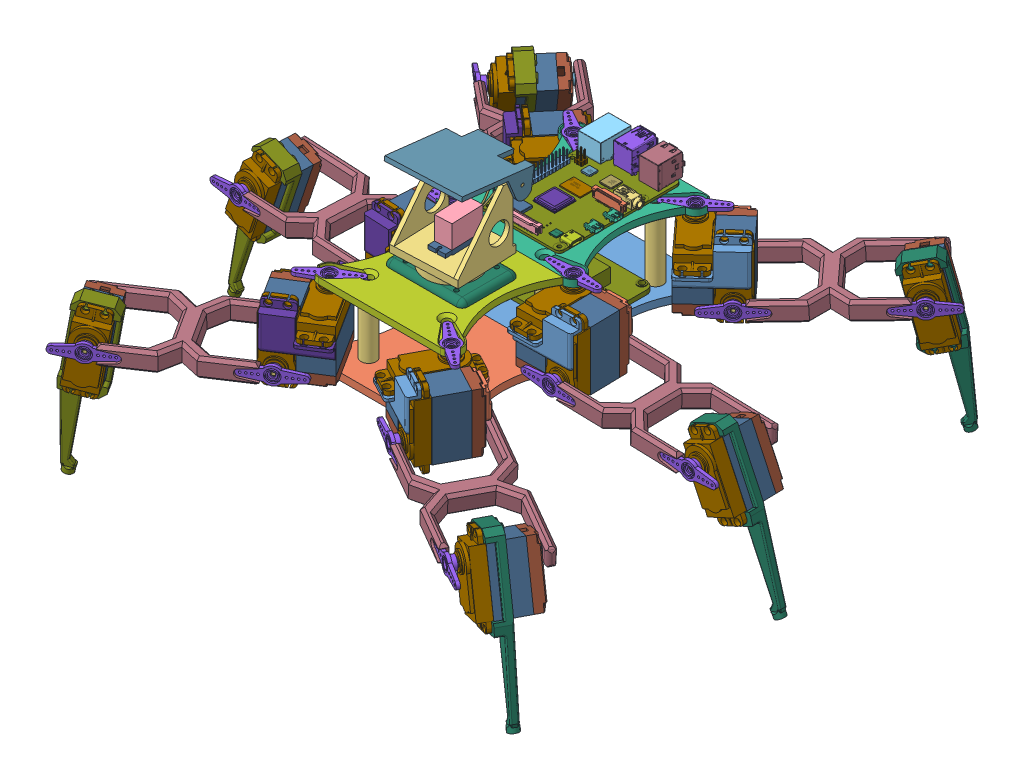
SolidWorks assembly 初号机, configuration 默认. Lengths in mm.
Overall size (454.39 273.32 390.58).
241 component instances, 55 part files, 149 mates.
Components (placement in the parent):
- bottom^初号机-1: bottom^初号机 [默认] at origin size (100 5 185) (virtual)
  - Основание нижнее^bottom_初号机-1: Основание нижнее^bottom_初号机 [默认] at origin size (100 5 100) (virtual)
  - Основание нижнее-0^bottom_初号机-1: Основание нижнее-0^bottom_初号机 [默认] at origin size (100 5 87.2) (virtual)
- 底板支柱-1: 底板支柱 [По умолчанию] at (-26.5949 5 115.9923) x (-0.996474 0 0.083904) z (-0.083904 0 -0.996474) size (10.4 45 10.4)
- 底板支柱-2: 底板支柱 [По умолчанию] at (-22.868 5 42.5) x (-0.515212 0 0.857063) z (-0.857063 0 -0.515212) size (10.4 45 10.4)
- 底板支柱-3: 底板支柱 [По умолчанию] at (-26.5949 5 -30.9923) x (0.99992 0 0.012686) z (-0.012686 0 0.99992) size (10.4 45 10.4)
- 底板支柱-4: 底板支柱 [По умолчанию] at (27.1009 5 -30.1473) x (-0.03949 0 0.99922) z (-0.99922 0 -0.03949) size (10.4 45 10.4)
- 底板支柱-5: 底板支柱 [По умолчанию] at (22.868 5 42.5) x (-0.794557 0 0.607189) z (-0.607189 0 -0.794557) size (10.4 45 10.4)
- 底板支柱-6: 底板支柱 [По умолчанию] at (27.1009 5 115.1473) x (-0.645742 0 -0.763556) z (0.763556 0 -0.645742) size (10.4 45 10.4)
- 零件3^初号机-1: 零件3^初号机 [默认] at (19.1195 18 -11.2067) x (1 0 0) z (0 1 0) (virtual)
- 零件4^初号机-1: 零件4^初号机 [默认] at (0 5 0) x (1 0 0) z (0 1 0) (virtual)
- 零件5^初号机-1: 零件5^初号机 [默认] x (-1 0 0) z (0 -1 0) (virtual)
- 底板转柱-1: 底板转柱 [По умолчанию] at (-42.5 0.3 -42.5) x (0.027977 0 0.999609) z (-0.999609 0 0.027977) size (6.4 6 6.4)
- 轴承-1: 轴承 [По умолчанию] at (-42.5 3 -42.5) size (8 2.5 8)
- 底板转柱-2: 底板转柱 [По умолчанию] at (42.5 0.5 -42.5) x (0.999982 0 -0.006066) z (0.006066 0 0.999982) size (6.4 6 6.4)
- 轴承-2: 轴承 [По умолчанию] at (42.5 3 -42.5) size (8 2.5 8)
- 底板转柱-3: 底板转柱 [По умолчанию] at (42.5 2.5 42.5) size (6.4 6 6.4)
- 轴承-3: 轴承 [По умолчанию] at (42.5 5 42.5) size (8 2.5 8)
- 底板转柱-4: 底板转柱 [По умолчанию] at (42.5 0.5 127.5) x (0.985953 0 0.167025) z (-0.167025 0 0.985953) size (6.4 6 6.4)
- 轴承-4: 轴承 [По умолчанию] at (42.5 3 127.5) size (8 2.5 8)
- 底板转柱-5: 底板转柱 [По умолчанию] at (-42.5 0.3 127.5) x (0.666115 0 -0.745849) z (0.745849 0 0.666115) size (6.4 6 6.4)
- 轴承-5: 轴承 [По умолчанию] at (-42.5 3 42.5) size (8 2.5 8)
- 底板转柱-6: 底板转柱 [По умолчанию] at (-42.5 0.5 42.5) x (0.831911 0 -0.55491) z (0.55491 0 0.831911) size (6.4 6 6.4)
- 轴承-6: 轴承 [По умолчанию] at (-42.5 3 127.5) size (8 2.5 8)
- top(3)-1: top(3) [默认] at (-10.4042 60.8113 -78.0074) size (100 5.41 185)
  - top(3)^top(3)-2: top(3)^top(3) [默认] at (10.4042 -10.8113 28.0074) size (100 5.41 185) (virtual)
    - ^top(3)_top(3)-1: ^top(3)_top(3) [默认] at origin size (100 5.41 100)
      - Основание нижнее^_top(3)_top(3)-1: Основание нижнее^_top(3)_top(3) [默认] at origin size (100 5.41 100) (virtual)
    - _private_var_mobile_Containers_Data_Application_327FD876-EF9E-4CCE-9D75-9D16AF0753A7_tmp_B33AE067-E3AF-4F21-8502-7502B160869B.tmp(2)^top(3)_top(3)-1: _private_var_mobile_Containers_Data_Application_327FD876-EF9E-4CCE-9D75-9D16AF0753A7_tmp_B33AE067-E3AF-4F21-8502-7502B160869B.tmp(2)^top(3)_top(3) [默认] at origin size (100 5.41 85.65) (virtual)
- 舵机配件-3: 舵机配件 [По умолчанию] at (42.5 51.5 -42.5) x (0.783045 0 -0.621965) z (0.621965 0 0.783045) size (38 5.5 11.95)
- 舵机配件-4: 舵机配件 [По умолчанию] at (-42.5 51.5 -42.5) x (0.81018 0 0.586182) z (-0.586182 0 0.81018) size (38 5.5 11.95)
- 舵机配件-5: 舵机配件 [По умолчанию] at (-42.5 51.5 42.5) size (38 5.5 11.95)
- 舵机配件-6: 舵机配件 [По умолчанию] at (42.5 51.5 127.5) x (0.780043 0 0.625726) z (-0.625726 0 0.780043) size (38 5.5 11.95)
- 舵机配件-7: 舵机配件 [По умолчанию] at (-42.5 51.5 127.5) x (0.81018 0 -0.586182) z (0.586182 0 0.81018) size (38 5.5 11.95)
- 舵机配件-8: 舵机配件 [По умолчанию] at (42.5 51.5 42.5) x (-1 0 0) z (0 0 -1) size (38 5.5 11.95)
- Servo MG955-1: Servo MG955 [По умолчанию] at (-37.0524 34.5 136.0346) x (0.538039 0 0.84292) z (-0.84292 0 0.538039) size (54.05 45.1 20.2)
  - MG995前板-1: MG995前板 [По умолчанию] at origin size (54.05 13 19.8)
  - MG995中板-1: MG995中板 [По умолчанию] at (-0.05 -20.65 0) size (40.75 26.65 20.2)
  - MG995后板-1: MG995后板 [По умолчанию] at (-0.04 -28.1 0) size (40.73 8.25 20.2)
  - MG995齿轮-1: MG995齿轮 [По умолчанию] at (-10.125 13 0) size (6 4 6)
- 腿2-1: 腿2 [默认] at (185.4542 10.3474 -70.0497) x (0.896519 0.429402 -0.108939) z (0.120626 0 0.992698) size (139.95 134.21 56.85) (flexible)
  - Servo MG955-1: Servo MG955 [По умолчанию] at (-38.7357 8.5073 125.6329) x (-0.019851 -0.998955 0.041163) z (-0.995744 0.016048 -0.090749) size (54.05 45.1 20.2)
    - MG995前板-1: MG995前板 [По умолчанию] at origin size (54.05 13 19.8)
    - MG995中板-1: MG995中板 [По умолчанию] at (-0.05 -20.65 0) size (40.75 26.65 20.2)
    - MG995后板-1: MG995后板 [По умолчанию] at (-0.04 -28.1 0) size (40.73 8.25 20.2)
    - MG995齿轮-1: MG995齿轮 [По умолчанию] at (-10.125 13 0) size (6 4 6)
  - 腿上部-1: 腿上部 [По умолчанию] at (-122.3446 70.8812 116.3257) x (0.092332 -0.044042 -0.994754) z (-0.471738 -0.881726 -0.004749) size (56.54 115.05 13)
  - 舵机配件-1: 舵机配件 [По умолчанию] at (-40.0646 19.3492 142.1316) x (0.877134 -0.469818 0.099535) z (-0.471738 -0.881726 -0.004749) size (38 5.5 11.95)
  - 腿部转柱-1: 腿部转柱 [По умолчанию] at (-35.2687 17.0635 90.0982) x (0.012514 -0.998891 0.045387) z (-0.99565 -0.016639 -0.091679) size (6.4 7 6.4)
  - 轴承-1: 轴承 [По умолчанию] at (-35.7304 17.2837 95.072) x (0.994989 -0.034408 0.093878) z (0.038362 0.998437 -0.040644) size (8 2.5 8)
  - 舵机配件-2: 舵机配件 [По умолчанию] at (-123.4791 64.0283 132.6658) x (-0.877134 0.469818 -0.099535) z (0.471738 0.881726 0.004749) size (38 5.5 11.95)
  - Servo MG955-2: Servo MG955 [По умолчанию] at (-117.6015 72.4449 115.7505) x (0.429402 0.903113 0) z (0.898618 -0.427265 0.099649) size (54.05 45.1 20.2)
    - MG995前板-1: MG995前板 [По умолчанию] at origin size (54.05 13 19.8)
    - MG995中板-1: MG995中板 [По умолчанию] at (-0.05 -20.65 0) size (40.75 26.65 20.2)
    - MG995后板-1: MG995后板 [По умолчанию] at (-0.04 -28.1 0) size (40.73 8.25 20.2)
    - MG995齿轮-1: MG995齿轮 [По умолчанию] at (-10.125 13 0) size (6 4 6)
  - 轴承-2: 轴承 [По умолчанию] at (-118.8546 61.8223 82.8713) x (0.932326 -0.346965 0.101899) z (-0.349632 -0.936844 0.009025) size (8 2.5 8)
  - 腿部转柱-2: 腿部转柱 [По умолчанию] at (-118.6238 61.7122 80.3845) x (0.762634 0.645451 0.04221) z (0.640206 -0.762531 0.093184) size (6.4 7 6.4)
  - 腿2下部-1: 腿2下部 [По умолчанию] at (-39.3424 -60.1376 124.0075) x (-0.995744 0.016048 -0.090749) z (0.089994 -0.042789 -0.995023) size (25.9 109 11.67)
- 腿1-2: 腿1 [默认] at (-98.6355 -7.7779 36.8806) x (0.936595 0.175518 -0.303287) z (0.30807 0 0.951364) size (162.83 108.04 56.85) (flexible)
  - 腿1下部-1: 腿1下部 [По умолчанию] at (-105.262 -37.9443 138.365) x (0.916143 -0.313809 -0.24941) z (0.248278 -0.044264 0.967677) size (25.9 109 11.67)
  - Servo MG955-1: Servo MG955 [По умолчанию] at (-79.2817 26.202 151.6846) x (-0.314705 -0.948454 0.037359) z (-0.916143 0.313809 0.24941) size (54.05 45.1 20.2)
    - MG995前板-1: MG995前板 [По умолчанию] at origin size (54.05 13 19.8)
    - MG995中板-1: MG995中板 [По умолчанию] at (-0.05 -20.65 0) size (40.75 26.65 20.2)
    - MG995后板-1: MG995后板 [По умолчанию] at (-0.04 -28.1 0) size (40.73 8.25 20.2)
    - MG995齿轮-1: MG995齿轮 [По умолчанию] at (-10.125 13 0) size (6 4 6)
  - 腿上部-1: 腿上部 [По умолчанию] at (17.5111 13.6079 127.2377) x (-0.250822 0.044688 -0.967001) z (0.165142 0.986266 0.002744) size (56.54 115.05 13)
  - 舵机配件-1: 舵机配件 [По умолчанию] at (-71.8746 35.0526 167.7568) x (-0.954508 0.159123 0.252178) z (0.165142 0.986266 0.002744) size (38 5.5 11.95)
  - 腿部转柱-1: 腿部转柱 [По умолчанию] at (-84.9572 37.3839 117.1692) x (0.343653 -0.929759 -0.132104) z (-0.904981 -0.365447 0.217846) size (6.4 7 6.4)
  - 轴承-1: 轴承 [По умолчанию] at (-83.7031 37.1604 122.0042) x (0.921354 0.317477 -0.22431) z (-0.296976 0.947212 0.120804) size (8 2.5 8)
  - 舵机配件-2: 舵机配件 [По умолчанию] at (18.8981 19.9202 143.775) x (0.954508 -0.159123 -0.252178) z (-0.165142 -0.986266 -0.002744) size (38 5.5 11.95)
  - Servo MG955-2: Servo MG955 [По умолчанию] at (16.4545 30.6405 127.3245) x (0.175518 0.984476 0) z (0.952655 -0.169844 -0.252193) size (54.05 45.1 20.2)
    - MG995前板-1: MG995前板 [По умолчанию] at origin size (54.05 13 19.8)
    - MG995中板-1: MG995中板 [По умолчанию] at (-0.05 -20.65 0) size (40.75 26.65 20.2)
    - MG995后板-1: MG995后板 [По умолчанию] at (-0.04 -28.1 0) size (40.73 8.25 20.2)
    - MG995齿轮-1: MG995齿轮 [По умолчанию] at (-10.125 13 0) size (6 4 6)
  - 轴承-2: 轴承 [По умолчанию] at (6.3398 22.1576 95.3702) x (0.967999 0.003155 -0.250935) z (-0.008163 -0.998996 -0.04405) size (8 2.5 8)
  - 腿部转柱-2: 腿部转柱 [По умолчанию] at (5.7128 22.2693 92.9526) x (0.482761 0.871623 -0.084939) z (0.839065 -0.488135 -0.240196) size (6.4 7 6.4)
- 固定件1-1: 固定件1 [默认] at (-26.1167 13.85 153.1669) x (0.84292 0 -0.538039) z (0.538039 0 0.84292) size (39.3 28.12 13.1)
- 固定件2-1: 固定件2 [默认] at (-48.0418 13.85 118.8179) x (-0.84292 0 0.538039) z (-0.538039 0 -0.84292) size (39.6 20.62 9.9)
- 腿1-3: 腿1 [默认] at (-64.9276 -7.7779 -61.7117) x (0.984049 0.175518 0.029006) z (-0.029463 0 0.999566) size (162.83 108.04 56.85) (flexible)
  - 腿1下部-1: 腿1下部 [По умолчанию] at (-122.8705 -29.575 103.698) x (0.873531 -0.486444 0.017789) z (-0.018522 0.003302 0.999823) size (25.9 109 11.67)
  - Servo MG955-1: Servo MG955 [По умолчанию] at (-89.542 30.1741 120.621) x (-0.486417 -0.873706 -0.006125) z (-0.873531 0.486444 -0.017789) size (54.05 45.1 20.2)
    - MG995前板-1: MG995前板 [По умолчанию] at origin size (54.05 13 19.8)
    - MG995中板-1: MG995中板 [По умолчанию] at (-0.05 -20.65 0) size (40.75 26.65 20.2)
    - MG995后板-1: MG995后板 [По умолчанию] at (-0.04 -28.1 0) size (40.73 8.25 20.2)
    - MG995齿轮-1: MG995齿轮 [По умолчанию] at (-10.125 13 0) size (6 4 6)
  - 腿上部-1: 腿上部 [По умолчанию] at (11.4606 14.6177 123.4759) x (0.0159 -0.002817 -0.99987) z (0.182086 0.983283 0.000126) size (56.54 115.05 13)
  - 舵机配件-1: 舵机配件 [По умолчанию] at (-84.9319 39.0765 137.68) x (-0.983108 0.182056 -0.018813) z (0.182086 0.983283 0.000126) size (38 5.5 11.95)
  - 腿部转柱-1: 腿部转柱 [По умолчанию] at (-84.0628 38.9222 85.3836) x (0.36033 -0.932787 0.008358) z (-0.932689 -0.360416 -0.013817) size (6.4 7 6.4)
  - 轴承-1: 轴承 [По умолчанию] at (-84.1423 38.9363 90.383) x (0.949878 0.312297 0.014226) z (-0.312217 0.94998 -0.007641) size (8 2.5 8)
  - 舵机配件-2: 舵机配件 [По умолчанию] at (8.5607 21.7632 139.4692) x (0.983108 -0.182056 0.018813) z (-0.182086 -0.983283 -0.000126) size (38 5.5 11.95)
  - Servo MG955-2: Servo MG955 [По умолчанию] at (10.6526 31.6749 122.4722) x (0.175518 0.984476 0) z (0.984302 -0.175487 0.018814) size (54.05 45.1 20.2)
    - MG995前板-1: MG995前板 [По умолчанию] at origin size (54.05 13 19.8)
    - MG995中板-1: MG995中板 [По умолчанию] at (-0.05 -20.65 0) size (40.75 26.65 20.2)
    - MG995后板-1: MG995后板 [По умолчанию] at (-0.04 -28.1 0) size (40.73 8.25 20.2)
    - MG995齿轮-1: MG995齿轮 [По умолчанию] at (-10.125 13 0) size (6 4 6)
  - 轴承-2: 轴承 [По умолчанию] at (9.3537 21.6227 89.4182) x (0.99987 -0.002633 0.015908) z (-0.002677 -0.999993 0.002774) size (8 2.5 8)
  - 腿部转柱-2: 腿部转柱 [По умолчанию] at (9.3935 21.6157 86.9186) x (0.493644 0.869647 0.0054) z (0.869519 -0.493665 0.015218) size (6.4 7 6.4)
- 腿1-4: 腿1 [默认] at (-0.0766 -7.7779 -140.2922) x (0.783275 0.175518 0.596384) z (-0.605788 0 0.795626) size (162.83 108.04 56.85) (flexible)
  - 腿1下部-1: 腿1下部 [По умолчанию] at (-136.8171 -32.3512 98.6616) x (0.761205 -0.647085 0.042994) z (-0.048987 0.008734 0.998761) size (25.9 109 11.67)
  - Servo MG955-1: Servo MG955 [По умолчанию] at (-93.051 19.8026 116.8726) x (-0.646658 -0.762368 -0.025051) z (-0.761205 0.647085 -0.042994) size (54.05 45.1 20.2)
    - MG995前板-1: MG995前板 [По умолчанию] at origin size (54.05 13 19.8)
    - MG995中板-1: MG995中板 [По умолчанию] at (-0.05 -20.65 0) size (40.75 26.65 20.2)
    - MG995后板-1: MG995后板 [По умолчанию] at (-0.04 -28.1 0) size (40.73 8.25 20.2)
    - MG995齿轮-1: MG995齿轮 [По умолчанию] at (-10.125 13 0) size (6 4 6)
  - 腿上部-1: 腿上部 [По умолчанию] at (11.7079 15.0972 122.9854) x (0.046329 -0.008574 -0.998889) z (0.060434 0.998156 -0.005764) size (56.54 115.05 13)
  - 舵机配件-1: 舵机配件 [По умолчанию] at (-87.3364 27.6701 134.1052) x (-0.996969 0.060076 -0.049425) z (0.060434 0.998156 -0.005764) size (38 5.5 11.95)
  - 腿部转柱-1: 腿部转柱 [По умолчанию] at (-84.8752 27.2193 81.8612) x (0.360008 -0.932622 0.024702) z (-0.931798 -0.360753 -0.040121) size (6.4 7 6.4)
  - 轴承-1: 轴承 [По умолчанию] at (-85.1068 27.2622 86.8557) x (0.948971 0.312642 0.04133) z (-0.311941 0.949832 -0.02262) size (8 2.5 8)
  - 舵机配件-2: 舵机配件 [По умолчанию] at (7.4743 21.9569 138.8055) x (0.996969 -0.060076 0.049425) z (-0.060434 -0.998156 0.005764) size (38 5.5 11.95)
  - Servo MG955-2: Servo MG955 [По умолчанию] at (10.0842 31.7762 121.8265) x (0.175518 0.984476 0) z (0.983257 -0.1753 0.04976) size (54.05 45.1 20.2)
    - MG995前板-1: MG995前板 [По умолчанию] at origin size (54.05 13 19.8)
    - MG995中板-1: MG995中板 [По умолчанию] at (-0.05 -20.65 0) size (40.75 26.65 20.2)
    - MG995后板-1: MG995后板 [По умолчанию] at (-0.04 -28.1 0) size (40.73 8.25 20.2)
    - MG995齿轮-1: MG995齿轮 [По умолчанию] at (-10.125 13 0) size (6 4 6)
  - 轴承-2: 轴承 [По умолчанию] at (9.7905 21.5279 88.8035) x (0.998923 -0.002259 0.04635) z (-0.002653 -0.999961 0.00846) size (8 2.5 8)
  - 腿部转柱-2: 腿部转柱 [По умолчанию] at (9.9064 21.5064 86.3063) x (0.493158 0.869803 0.015407) z (0.868705 -0.493324 0.044525) size (6.4 7 6.4)
- Servo MG955-2: Servo MG955 [По умолчанию] at (-42.9887 34.5 52.6132) x (-0.048264 0 0.998835) z (-0.998835 0 -0.048264) size (54.05 45.1 20.2)
  - MG995前板-1: MG995前板 [По умолчанию] at origin size (54.05 13 19.8)
  - MG995中板-1: MG995中板 [По умолчанию] at (-0.05 -20.65 0) size (40.75 26.65 20.2)
  - MG995后板-1: MG995后板 [По умолчанию] at (-0.04 -28.1 0) size (40.73 8.25 20.2)
  - MG995齿轮-1: MG995齿轮 [По умолчанию] at (-10.125 13 0) size (6 4 6)
- 固定件1-2: 固定件1 [默认] at (-43.9696 13.85 72.9145) x (0.998835 0 0.048264) z (-0.048264 0 0.998835) size (39.3 28.12 13.1)
- 固定件2-2: 固定件2 [默认] at (-42.0029 13.85 32.212) x (-0.998835 0 -0.048264) z (0.048264 0 -0.998835) size (39.6 20.62 9.9)
- 固定件1-3: 固定件1 [默认] at (-62.1289 13.85 -19.2211) x (0.764496 0 0.644628) z (-0.644628 0 0.764496) size (39.3 28.12 13.1)
- 固定件2-3: 固定件2 [默认] at (-35.8603 13.85 -50.3743) x (-0.764496 0 -0.644628) z (0.644628 0 -0.764496) size (39.6 20.62 9.9)
- Servo MG955-4: Servo MG955 [По умолчанию] at (37.7593 34.5 136.4466) x (-0.468216 0 0.883614) z (-0.883614 0 -0.468216) size (54.05 45.1 20.2)
  - MG995前板-1: MG995前板 [По умолчанию] at origin size (54.05 13 19.8)
  - MG995中板-1: MG995中板 [По умолчанию] at (-0.05 -20.65 0) size (40.75 26.65 20.2)
  - MG995后板-1: MG995后板 [По умолчанию] at (-0.04 -28.1 0) size (40.73 8.25 20.2)
  - MG995齿轮-1: MG995齿轮 [По умолчанию] at (-10.125 13 0) size (6 4 6)
- 腿2-2: 腿2 [默认] at (207.5876 -39.0456 86.6973) x (0.593758 0.775503 0.214582) z (-0.339882 0 0.940468) size (139.95 134.21 56.85) (flexible)
  - Servo MG955-1: Servo MG955 [По умолчанию] at (10.6136 43.607 130.1862) x (-0.532766 -0.845059 0.045109) z (-0.841633 0.52353 -0.132553) size (54.05 45.1 20.2)
    - MG995前板-1: MG995前板 [По умолчанию] at origin size (54.05 13 19.8)
    - MG995中板-1: MG995中板 [По умолчанию] at (-0.05 -20.65 0) size (40.75 26.65 20.2)
    - MG995后板-1: MG995后板 [По умолчанию] at (-0.04 -28.1 0) size (40.73 8.25 20.2)
    - MG995齿轮-1: MG995齿轮 [По умолчанию] at (-10.125 13 0) size (6 4 6)
  - 腿上部-1: 腿上部 [По умолчанию] at (-33.1252 137.3491 116.9425) x (0.089867 -0.110779 -0.989774) z (-0.830304 -0.557158 -0.013028) size (56.54 115.05 13)
  - 舵机配件-1: 舵机配件 [По умолчанию] at (14.5051 54.0092 146.562) x (0.550255 -0.823277 0.139411) z (-0.830304 -0.557158 -0.013028) size (38 5.5 11.95)
  - 腿部转柱-1: 腿部转柱 [По умолчанию] at (19.1845 48.2464 94.7876) x (-0.419139 -0.905712 0.063315) z (-0.903463 0.409163 -0.127825) size (6.4 7 6.4)
  - 轴承-1: 轴承 [По умолчанию] at (18.7352 48.8003 99.7365) x (0.880874 -0.454894 0.130893) z (0.464742 0.883629 -0.056703) size (8 2.5 8)
  - 舵机配件-2: 舵机配件 [По умолчанию] at (-37.8235 132.3019 133.3042) x (-0.550255 0.823277 -0.139411) z (0.830304 0.557158 0.013028) size (38 5.5 11.95)
  - Servo MG955-2: Servo MG955 [По умолчанию] at (-28.4688 136.8483 116.4716) x (0.775503 0.631343 0) z (0.625124 -0.767864 0.140018) size (54.05 45.1 20.2)
    - MG995前板-1: MG995前板 [По умолчанию] at origin size (54.05 13 19.8)
    - MG995中板-1: MG995中板 [По умолчанию] at (-0.05 -20.65 0) size (40.75 26.65 20.2)
    - MG995后板-1: MG995后板 [По умолчанию] at (-0.04 -28.1 0) size (40.73 8.25 20.2)
    - MG995齿轮-1: MG995齿轮 [По умолчанию] at (-10.125 13 0) size (6 4 6)
  - 轴承-2: 轴承 [По умолчанию] at (-33.3235 126.7542 83.7591) x (0.689789 -0.709931 0.142088) z (-0.718412 -0.695504 0.012615) size (8 2.5 8)
  - 腿部转柱-2: 腿部转柱 [По умолчанию] at (-33.0988 126.4772 81.2846) x (0.964645 0.256904 0.058831) z (0.247759 -0.960067 0.12995) size (6.4 7 6.4)
  - 腿2下部-1: 腿2下部 [По умолчанию] at (-25.1983 -14.9669 128.8677) x (-0.841633 0.52353 -0.132553) z (0.0884 -0.108585 -0.990149) size (25.9 109 11.67)
- 镜向固定件1-1: 镜向固定件1 [默认] at (28.2428 13.85 154.406) x (-0.883614 0 -0.468216) z (0.468216 0 -0.883614) size (39.3 28.12 13.1)
- 镜向固定件2-1: 镜向固定件2 [默认] at (47.3226 13.85 118.3988) x (0.883614 0 0.468216) z (-0.468216 0 0.883614) size (39.6 20.62 9.9)
- Servo MG955-5: Servo MG955 [По умолчанию] at (42.7137 34.5 52.6227) x (0.021104 0 0.999777) z (-0.999777 0 0.021104) size (54.05 45.1 20.2)
  - MG995前板-1: MG995前板 [По умолчанию] at origin size (54.05 13 19.8)
  - MG995中板-1: MG995中板 [По умолчанию] at (-0.05 -20.65 0) size (40.75 26.65 20.2)
  - MG995后板-1: MG995后板 [По умолчанию] at (-0.04 -28.1 0) size (40.73 8.25 20.2)
  - MG995齿轮-1: MG995齿轮 [По умолчанию] at (-10.125 13 0) size (6 4 6)
- 镜向固定件1-2: 镜向固定件1 [默认] at (43.1426 13.85 72.9432) x (-0.999777 0 0.021104) z (-0.021104 0 -0.999777) size (39.3 28.12 13.1)
- 镜向固定件2-2: 镜向固定件2 [默认] at (42.2826 13.85 32.2023) x (0.999777 0 -0.021104) z (0.021104 0 0.999777) size (39.6 20.62 9.9)
- Servo MG955-6: Servo MG955 [По умолчанию] at (49.3266 34.5 -35.0225) x (0.674231 0 0.73852) z (-0.73852 0 0.674231) size (54.05 45.1 20.2)
  - MG995前板-1: MG995前板 [По умолчанию] at origin size (54.05 13 19.8)
  - MG995中板-1: MG995中板 [По умолчанию] at (-0.05 -20.65 0) size (40.75 26.65 20.2)
  - MG995后板-1: MG995后板 [По умолчанию] at (-0.04 -28.1 0) size (40.73 8.25 20.2)
  - MG995齿轮-1: MG995齿轮 [По умолчанию] at (-10.125 13 0) size (6 4 6)
- 腿2-3: 腿2 [默认] at (69.8042 -26.4289 -197.3993) x (0.735555 0.089531 -0.671523) z (0.674231 0 0.73852) size (139.95 134.21 56.85)
  - Servo MG955-1: Servo MG955 [По умолчанию] at (-3.8004 36.7708 115.337) x (0.142633 -0.989776 0) z (-0.989776 -0.142633 0) size (54.05 45.1 20.2)
    - MG995前板-1: MG995前板 [По умолчанию] at origin size (54.05 13 19.8)
    - MG995中板-1: MG995中板 [По умолчанию] at (-0.05 -20.65 0) size (40.75 26.65 20.2)
    - MG995后板-1: MG995后板 [По умолчанию] at (-0.04 -28.1 0) size (40.73 8.25 20.2)
    - MG995齿轮-1: MG995齿轮 [По умолчанию] at (-10.125 13 0) size (6 4 6)
  - 腿上部-1: 腿上部 [По умолчанию] at (-103.8372 57.4142 116.2692) x (0.002664 -0.000111 -0.999996) z (-0.041713 -0.99913 0) size (56.54 115.05 13)
  - 舵机配件-1: 舵机配件 [По умолчанию] at (-5.2446 46.7923 132.337) x (0.99913 -0.041713 0) z (-0.041713 -0.99913 0) size (38 5.5 11.95)
  - 腿部转柱-1: 腿部转柱 [По умолчанию] at (-5.1433 46.7881 80.0332) x (0.360472 -0.93277 0.001064) z (-0.932766 -0.360473 -0.002445) size (6.4 7 6.4)
  - 轴承-1: 轴承 [По умолчанию] at (-5.1566 46.7886 85.0332) x (0.949962 0.312356 0.002496) z (-0.312354 0.949965 -0.000938) size (8 2.5 8)
  - 舵机配件-2: 舵机配件 [По умолчанию] at (-100.2607 50.7592 132.337) x (-0.99913 0.041713 0) z (0.041713 0.99913 0) size (38 5.5 11.95)
  - Servo MG955-2: Servo MG955 [По умолчанию] at (-99.3542 60.8435 115.337) x (0.089531 0.995984 0) z (0.995984 -0.089531 0) size (54.05 45.1 20.2)
    - MG995前板-1: MG995前板 [По умолчанию] at origin size (54.05 13 19.8)
    - MG995中板-1: MG995中板 [По умолчанию] at (-0.05 -20.65 0) size (40.75 26.65 20.2)
    - MG995后板-1: MG995后板 [По умолчанию] at (-0.04 -28.1 0) size (40.73 8.25 20.2)
    - MG995齿轮-1: MG995齿轮 [По умолчанию] at (-10.125 13 0) size (6 4 6)
  - 轴承-2: 轴承 [По умолчанию] at (-100.1245 50.7535 82.2797) x (0.999993 -0.002573 0.002664) z (-0.002573 -0.999997 0.000104) size (8 2.5 8)
  - 腿部转柱-2: 腿部转柱 [По умолчанию] at (-100.1178 50.7532 79.7797) x (0.493614 0.86968 0.001218) z (0.869677 -0.493615 0.002372) size (6.4 7 6.4)
  - 腿2下部-1: 腿2下部 [По умолчанию] at (6.319 -30.997 110.837) x (-0.989776 -0.142633 0) z (0 0 -1) size (25.9 109 11.67)
- 镜向固定件1-3: 镜向固定件1 [默认] at (63.0303 13.85 -20.0121) x (-0.73852 0 0.674231) z (-0.674231 0 -0.73852) size (39.3 28.12 13.1)
- 镜向固定件2-3: 镜向固定件2 [默认] at (35.5554 13.85 -50.1068) x (0.73852 0 -0.674231) z (0.674231 0 0.73852) size (39.6 20.62 9.9)
- Servo MG955-7: Servo MG955 [По умолчанию] at (-49.0269 34.5 -34.7595) x (-0.644628 0 0.764496) z (-0.764496 0 -0.644628) size (54.05 45.1 20.2)
  - MG995前板-1: MG995前板 [По умолчанию] at origin size (54.05 13 19.8)
  - MG995中板-1: MG995中板 [По умолчанию] at (-0.05 -20.65 0) size (40.75 26.65 20.2)
  - MG995后板-1: MG995后板 [По умолчанию] at (-0.04 -28.1 0) size (40.73 8.25 20.2)
  - MG995齿轮-1: MG995齿轮 [По умолчанию] at (-10.125 13 0) size (6 4 6)
- 云台2号机 -1: 云台2号机  [默认] at (15.9909 62.7925 82.7589) x (0.932039 0 0.362358) z (-0.362358 0 0.932039) size (66.68 65.32 69.63) (flexible)
  - 云台2-1: 云台2 [默认] at (-14.0921 2.7075 7.8833) x (-0.39965 0 -0.916668) z (0.916668 0 -0.39965) size (49.22 53.71 51)
  - servo motor assembley-1: servo motor assembley [默认] at (-30.4131 17.0295 -4.0404) x (-0.39965 0 -0.916668) z (0 -1 0) size (45.87 13.05 32.83)
    - servo motor assembley(2)^servo motor assembley-1: servo motor assembley(2)^servo motor assembley [默认] at (-1.1752 7.1939 -5.155) size (45.87 13.05 32.83) (virtual)
      - lower cover^servo motor assembley(2)_servo motor assembley-1: lower cover^servo motor assembley(2)_servo motor assembley [默认] at (-10.9275 3.0017 -4.223) size (22.5 11.8 15.9) (virtual)
      - motor^servo motor assembley(2)_servo motor assembley-1: motor^servo motor assembley(2)_servo motor assembley [默认] at (-9.5275 2.9783 11.077) x (-0.99999 -0.004374 0) z (0 0 -1) size (7.82 7.82 13.51) (virtual)
      - feedback potentiometer^servo motor assembley(2)_servo motor assembley-1: feedback potentiometer^servo motor assembley(2)_servo motor assembley [默认] at (-9.0275 3.0017 11.177) x (-1 0 0) z (0 0 -1) size (7.71 7.36 13.7) (virtual)
      - 复件 (2) ^servo motor assembley(2)_servo motor assembley-1: 复件 (2) ^servo motor assembley(2)_servo motor assembley [默认] at (-9.517 2.6091 11.927) x (0.924877 -0.380266 0) z (0 0 1) size (10 10 5.7) (virtual)
      - 复件 (3) ^servo motor assembley(2)_servo motor assembley-1: 复件 (3) ^servo motor assembley(2)_servo motor assembley [默认] at (-9.3501 4.3681 11.477) x (0.966834 -0.255406 0) z (0 0 1) size (3.22 3.24 1.95) (virtual)
      - 复件 (4) ^servo motor assembley(2)_servo motor assembley-1: 复件 (4) ^servo motor assembley(2)_servo motor assembley [默认] at (-11.9047 8.7845 13.077) x (0.603146 0.797631 0) z (0 0 1) size (8.02 8.02 12.7) (virtual)
      - upper cover^servo motor assembley(2)_servo motor assembley-1: upper cover^servo motor assembley(2)_servo motor assembley [默认] at (-10.9275 3.0017 11.677) x (-1 0 0) z (0 0 1) size (31.9 11.8 10.8) (virtual)
      - 复件 (6) ^servo motor assembley(2)_servo motor assembley-1: 复件 (6) ^servo motor assembley(2)_servo motor assembley [默认] at (-10.9275 3.0017 -3.723) size (11.69 9.5 1.25) (virtual)
      - 复件 (7) ^servo motor assembley(2)_servo motor assembley-1: 复件 (7) ^servo motor assembley(2)_servo motor assembley [默认] at (-10.9275 -2.8983 -4.223) x (-1 0 0) z (0 -1 0) size (34.01 15.81 10.46) (virtual)
  - servo motor assembley-2: servo motor assembley [默认] at (-18.4343 36.679 4.6244) x (0.395273 0.147601 0.906627) z (-0.916668 0 0.39965) size (45.87 13.05 32.83)
    - servo motor assembley(2)^servo motor assembley-1: servo motor assembley(2)^servo motor assembley [默认] at (-1.1752 7.1939 -5.155) size (45.87 13.05 32.83) (virtual)
      - lower cover^servo motor assembley(2)_servo motor assembley-1: lower cover^servo motor assembley(2)_servo motor assembley [默认] at (-10.9275 3.0017 -4.223) size (22.5 11.8 15.9) (virtual)
      - motor^servo motor assembley(2)_servo motor assembley-1: motor^servo motor assembley(2)_servo motor assembley [默认] at (-9.5275 2.9783 11.077) x (-0.99999 -0.004374 0) z (0 0 -1) size (7.82 7.82 13.51) (virtual)
      - feedback potentiometer^servo motor assembley(2)_servo motor assembley-1: feedback potentiometer^servo motor assembley(2)_servo motor assembley [默认] at (-9.0275 3.0017 11.177) x (-1 0 0) z (0 0 -1) size (7.71 7.36 13.7) (virtual)
      - 复件 (2) ^servo motor assembley(2)_servo motor assembley-1: 复件 (2) ^servo motor assembley(2)_servo motor assembley [默认] at (-9.517 2.6091 11.927) x (0.924877 -0.380266 0) z (0 0 1) size (10 10 5.7) (virtual)
      - 复件 (3) ^servo motor assembley(2)_servo motor assembley-1: 复件 (3) ^servo motor assembley(2)_servo motor assembley [默认] at (-9.3501 4.3681 11.477) x (0.966834 -0.255406 0) z (0 0 1) size (3.22 3.24 1.95) (virtual)
      - 复件 (4) ^servo motor assembley(2)_servo motor assembley-1: 复件 (4) ^servo motor assembley(2)_servo motor assembley [默认] at (-11.9047 8.7845 13.077) x (0.603146 0.797631 0) z (0 0 1) size (8.02 8.02 12.7) (virtual)
      - upper cover^servo motor assembley(2)_servo motor assembley-1: upper cover^servo motor assembley(2)_servo motor assembley [默认] at (-10.9275 3.0017 11.677) x (-1 0 0) z (0 0 1) size (31.9 11.8 10.8) (virtual)
      - 复件 (6) ^servo motor assembley(2)_servo motor assembley-1: 复件 (6) ^servo motor assembley(2)_servo motor assembley [默认] at (-10.9275 3.0017 -3.723) size (11.69 9.5 1.25) (virtual)
      - 复件 (7) ^servo motor assembley(2)_servo motor assembley-1: 复件 (7) ^servo motor assembley(2)_servo motor assembley [默认] at (-10.9275 -2.8983 -4.223) x (-1 0 0) z (0 -1 0) size (34.01 15.81 10.46) (virtual)
  - 舵机配件1-1: 舵机配件1 [默认] at (-43.3377 43.2875 2.8575) x (0.396563 -0.124052 0.909587) z (-0.916668 0 0.39965) size (19.32 8.68 3.3)
  - 云台3-1: 云台3 [默认] at (-18.1026 56.3798 7.358) x (-0.916668 0 0.39965) z (-0.395273 -0.147601 -0.906627) size (51.95 18.16 57)
  - 云台1-1: 云台1 [默认] at (-14.0921 -3.7925 7.8833) x (0.932039 0 -0.362358) z (-0.362358 0 -0.932039) size (55 7 40)
  - 舵机配件1-2: 舵机配件1 [默认] at (-10.5991 -3.7925 14.2363) x (0.481797 0 0.876283) z (0 -1 0) size (19.32 8.68 3.3)
- rpi4b-1: rpi4b [默认] at (-23.3348 53.8739 -11.1948) x (0 0 -1) z (1 0 0) size (89 19.92 58.4)
  - rpi4b(2)^rpi4b-1: rpi4b(2)^rpi4b [默认] at (-6.5308 1.9261 23.3348) size (89 19.92 58.4) (virtual)
    - PCB, RPi4ModelB^rpi4b(2)_rpi4b-1: PCB, RPi4ModelB^rpi4b(2)_rpi4b [默认] at origin size (85 1.6 56) (virtual)
    - Broadcom BCM2711B0 CPU, RPi4ModelB^rpi4b(2)_rpi4b-1: Broadcom BCM2711B0 CPU, RPi4ModelB^rpi4b(2)_rpi4b [默认] at (-13.25 0.8 -4.5) size (15 2.3 15) (virtual)
    - 2.54 mm DUPONT MALE PIN HEADER, POE, 2X2, RPi4ModelB^rpi4b(2)_rpi4b-1: 2.54 mm DUPONT MALE PIN HEADER, POE, 2X2, RPi4ModelB^rpi4b(2)_rpi4b [默认] at (19 0.8 -18.36) size (5.08 11.3 5.08) (virtual)
    - 2.54 mm DUPONT MALE PIN HEADER, IO, 2X20, RPi4ModelB^rpi4b(2)_rpi4b-1: 2.54 mm DUPONT MALE PIN HEADER, IO, 2X20, RPi4ModelB^rpi4b(2)_rpi4b [默认] at (-10 0.8 -24.5) size (50.8 11.3 5.08) (virtual)
    - Camera Connector, RPi4ModelB^rpi4b(2)_rpi4b-1: Camera Connector, RPi4ModelB^rpi4b(2)_rpi4b [默认] at (4 0.8 16.5) x (0 0 -1) z (1 0 0) size (22.4 5.68 5.07) (virtual)
    - Microphone Plug, RPi4ModelB^rpi4b(2)_rpi4b-1: Microphone Plug, RPi4ModelB^rpi4b(2)_rpi4b [默认] at (11.5 0.8 21.65) size (7.23 7.55 15) (virtual)
    - Display Connector, RPi4ModelB^rpi4b(2)_rpi4b-1: Display Connector, RPi4ModelB^rpi4b(2)_rpi4b [默认] at (-38.5 0.8 0) x (0 0 1) z (-1 0 0) size (22.4 5.68 5.07) (virtual)
    - Gigabit Ethernet Port, RPi4ModelB^rpi4b(2)_rpi4b-1: Gigabit Ethernet Port, RPi4ModelB^rpi4b(2)_rpi4b [默认] at (45.5 7.55 -17.75) x (0 0 -1) z (1 0 0) size (16.33 17.24 21.6) (virtual)
    - Female Micro HDMI Connector, RPi4ModelB^rpi4b(2)_rpi4b-1: Female Micro HDMI Connector, RPi4ModelB^rpi4b(2)_rpi4b [默认] at (-3 0.8 27.3875) size (6.5 3.51 7.5) (virtual)
    - Female Micro HDMI Connector, RPi4ModelB^rpi4b(2)_rpi4b-2: Female Micro HDMI Connector, RPi4ModelB^rpi4b(2)_rpi4b [默认] at (-16.5 0.8 27.3875) size (6.5 3.51 7.5) (virtual)
    - Female USB Type C Connector, RPi4ModelB^rpi4b(2)_rpi4b-1: Female USB Type C Connector, RPi4ModelB^rpi4b(2)_rpi4b [默认] at (-31.3 0.8 26.5419) size (8.94 3.96 7.9) (virtual)
    - 2X USB3.0 PORTS, RPi4ModelB^rpi4b(2)_rpi4b-1: 2X USB3.0 PORTS, RPi4ModelB^rpi4b(2)_rpi4b [默认] at (37.07 0.8 1) size (17.48 19.42 15.69) (virtual)
    - 91D77 D9WHV 778K, 4 GB LPDDR4 SDRAM, RPi4ModelB^rpi4b(2)_rpi4b-1: 91D77 D9WHV 778K, 4 GB LPDDR4 SDRAM, RPi4ModelB^rpi4b(2)_rpi4b [默认] at (2.25 0.8 -4.5) size (10 0.8 14.5) (virtual)
    - Cypress CYW43455 Wireless Module Cover, RPi4ModelB^rpi4b(2)_rpi4b-1: Cypress CYW43455 Wireless Module Cover, RPi4ModelB^rpi4b(2)_rpi4b [默认] at (-30.5 0.8 -14.5) size (11 1.6 13) (virtual)
    - SD Card Slot, RPi4ModelB^rpi4b(2)_rpi4b-1: SD Card Slot, RPi4ModelB^rpi4b(2)_rpi4b [默认] at (-35.3 -0.8 0) x (0 0 -1) z (-1 0 0) size (11.95 1.45 11.4) (virtual)
    - VIA VL805 PCIe USB 3.0 controller, RPi4ModelB^rpi4b(2)_rpi4b-1: VIA VL805 PCIe USB 3.0 controller, RPi4ModelB^rpi4b(2)_rpi4b [默认] at (17.5 0.8 4) size (8.8 0.8 8.8) (virtual)
    - 2X USB2.0 PORTS, RPi4ModelB^rpi4b(2)_rpi4b-1: 2X USB2.0 PORTS, RPi4ModelB^rpi4b(2)_rpi4b [默认] at (37.065 0.65 19) size (17.87 19.17 15.35) (virtual)
    - Broadcom BCM54213PE Gigabit Ethernet Transceiver, RPi4ModelB^rpi4b(2)_rpi4b-1: Broadcom BCM54213PE Gigabit Ethernet Transceiver, RPi4ModelB^rpi4b(2)_rpi4b [默认] at (16.5 0.8 -10) size (6.8 1 6.8) (virtual)
    - MxL7704 Universal PMIC, RPi4ModelB^rpi4b(2)_rpi4b-1: MxL7704 Universal PMIC, RPi4ModelB^rpi4b(2)_rpi4b [默认] at (-32.5 0.8 16) size (5.4 0.8 5.4) (virtual)
